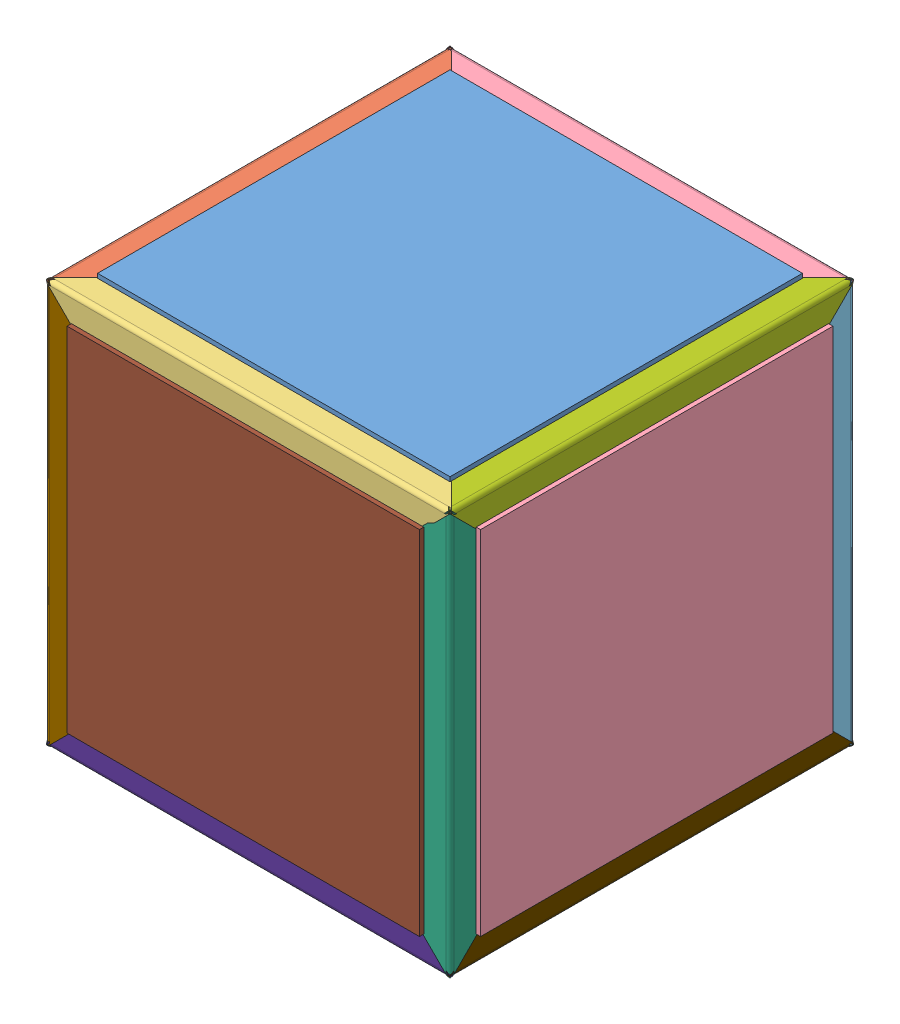
SolidWorks assembly cube_03, configuration cube03. Lengths in mm.
Overall size (150.49 150.49 150.49).
30 component instances, 30 part files, 92 mates.
Components (placement in the parent):
- pr^cube_03-28: pr^cube_03 [cube01] x (-1 0 0) z (0 0 1) size (128.27 1.59 128.27) (virtual)
- dr1^cube_03-55: dr1^cube_03 [cube01] at (-73.0546 73.66 0) x (0 -1 0) z (0 0 1) size (26.01 26.01 147.33) (virtual)
- dr2^cube_03-37: dr2^cube_03 [cube01] at (0 73.66 73.0546) x (0 -1 0) z (1 0 0) size (26.01 26.01 147.33) (virtual)
- dr3^cube_03-33: dr3^cube_03 [cube01] at (0 73.66 -73.0546) x (0 -1 0) z (-1 0 0) size (26.01 26.01 147.33) (virtual)
- br1^cube_03-49: br1^cube_03 [Default] at (0 48.26 -48.26) x (0 0 1) z (-1 0 0) size (50.8 50.8 89.41) (virtual)
- br2^cube_03-61: br2^cube_03 [Default] at (-48.26 48.26 0) size (50.8 50.8 89.41) (virtual)
- br3^cube_03-46: br3^cube_03 [Default] at (0 48.26 48.26) x (0 0 -1) z (1 0 0) size (50.8 50.8 89.41) (virtual)
- pg^cube_03-20: pg^cube_03 [cube01] x (0 -1 0) z (0 0 1) size (128.27 1.59 128.27) (virtual)
- dg1^cube_03-38: dg1^cube_03 [cube01] at (-73.66 0 73.0546) x (1 0 0) z (0 1 0) size (26.01 26.01 147.33) (virtual)
- dg2^cube_03-41: dg2^cube_03 [cube01] at (-73.66 -73.0546 0) size (26.01 26.01 147.33) (virtual)
- dg3^cube_03-34: dg3^cube_03 [cube01] at (-73.66 0 -73.0546) x (1 0 0) z (0 -1 0) size (26.01 26.01 147.33) (virtual)
- bg1^cube_03-47: bg1^cube_03 [Default] at (-48.26 -48.26 0) x (0 1 0) z (0 0 1) size (50.8 50.8 89.41) (virtual)
- bg2^cube_03-44: bg2^cube_03 [Default] at (-48.26 0 48.26) x (0 0 -1) z (0 1 0) size (50.8 50.8 89.41) (virtual)
- bg3^cube_03-40: bg3^cube_03 [Default] at (-48.26 0 -48.26) x (0 0 1) z (0 -1 0) size (50.8 50.8 89.41) (virtual)
- py^cube_03-21: py^cube_03 [cube01] at origin size (128.27 1.59 128.27) (virtual)
- dy1^cube_03-35: dy1^cube_03 [cube01] at (0 -73.66 -73.0546) x (0 1 0) z (1 0 0) size (26.01 26.01 147.33) (virtual)
- dy2^cube_03-39: dy2^cube_03 [cube01] at (0 -73.66 73.0546) x (0 1 0) z (-1 0 0) size (26.01 26.01 147.33) (virtual)
- dy3^cube_03-42: dy3^cube_03 [cube01] at (73.0546 -73.66 0) x (0 1 0) z (0 0 1) size (26.01 26.01 147.33) (virtual)
- by1^cube_03-41: by1^cube_03 [Default] at (0 -48.26 -48.26) x (0 0 1) z (1 0 0) size (50.8 50.8 89.41) (virtual)
- by2^cube_03-45: by2^cube_03 [Default] at (0 -48.26 48.26) x (0 0 -1) z (-1 0 0) size (50.8 50.8 89.41) (virtual)
- by3^cube_03-48: by3^cube_03 [Default] at (48.26 -48.26 0) x (-1 0 0) z (0 0 1) size (50.8 50.8 89.41) (virtual)
- po^cube_03-22: po^cube_03 [cube01] x (0 1 0) z (0 0 1) size (128.27 1.59 128.27) (virtual)
- do1^cube_03-36: do1^cube_03 [cube01] at (73.66 0 -73.0546) x (-1 0 0) z (0 1 0) size (26.01 26.01 147.33) (virtual)
- do2^cube_03-40: do2^cube_03 [cube01] at (73.66 0 73.0546) x (-1 0 0) z (0 -1 0) size (26.01 26.01 147.33) (virtual)
- do3^cube_03-47: do3^cube_03 [cube01] at (73.66 73.0546 0) x (-1 0 0) z (0 0 1) size (26.01 26.01 147.33) (virtual)
- bo1^cube_03-42: bo1^cube_03 [Default] at (48.26 0 -48.26) x (0 0 1) z (0 1 0) size (50.8 50.8 89.41) (virtual)
- bo2^cube_03-46: bo2^cube_03 [Default] at (48.26 0 48.26) x (0 0 -1) z (0 -1 0) size (50.8 50.8 89.41) (virtual)
- bo3^cube_03-62: bo3^cube_03 [Default] at (48.26 48.26 0) x (0 -1 0) z (0 0 1) size (50.8 50.8 89.41) (virtual)
- pc^cube_03-18: pc^cube_03 [cube01] x (-1 0 0) z (0 -1 0) size (128.27 1.59 128.27) (virtual)
- pb^cube_03-21: pb^cube_03 [cube01] x (-1 0 0) z (0 1 0) size (128.27 1.59 128.27) (virtual)
Mates (geometry in assembly coordinates):
- Coincident1: coincident anti-aligned: plane of pr^cube_03-28 through (64.135 73.66 -64.135) normal (0 -1 0); plane of br1^cube_03-49 through (-44.704 73.66 -48.26) normal (0 1 0)
- Coincident2: coincident anti-aligned: plane of pr^cube_03-28 through (64.135 73.66 -64.135) normal (0 -1 0); plane of br2^cube_03-61 through (-48.26 73.66 44.704) normal (0 1 0)
- Coincident3: coincident anti-aligned: plane of pr^cube_03-28 through (64.135 73.66 -64.135) normal (0 -1 0); plane of br3^cube_03-46 through (44.704 73.66 48.26) normal (0 1 0)
- Coincident4: coincident anti-aligned: plane of pr^cube_03-28 through (64.135 73.66 -64.135) normal (0 -1 0); plane of bo3^cube_03-62 through (48.26 73.66 44.704) normal (0 1 0)
- Coincident5: coincident anti-aligned: plane of pr^cube_03-28 through (64.135 73.66 -64.135) normal (0 -1 0); plane of dr3^cube_03-33 through (0 73.66 -146.7146) normal (0 1 0)
- Coincident6: coincident anti-aligned: plane of pr^cube_03-28 through (64.135 73.66 -64.135) normal (0 -1 0); plane of dr1^cube_03-55 through (-146.7146 73.66 0) normal (0 1 0)
- Coincident7: coincident anti-aligned: plane of pr^cube_03-28 through (64.135 73.66 -64.135) normal (0 -1 0); plane of do3^cube_03-47 through (-0.6054 73.66 0) normal (0 1 0)
- Coincident8: coincident anti-aligned: plane of pr^cube_03-28 through (64.135 73.66 -64.135) normal (0 -1 0); plane of dr2^cube_03-37 through (0 73.66 146.7146) normal (0 1 0)
- Coincident34: coincident anti-aligned: plane of pb^cube_03-21 through (64.135 -64.135 -73.66) normal (0 0 1); plane of by1^cube_03-41 through (44.704 -48.26 -73.66) normal (0 0 -1)
- Coincident35: coincident anti-aligned: plane of pb^cube_03-21 through (64.135 -64.135 -73.66) normal (0 0 1); plane of bo1^cube_03-42 through (48.26 44.704 -73.66) normal (0 0 -1)
- Coincident36: coincident anti-aligned: plane of pb^cube_03-21 through (64.135 -64.135 -73.66) normal (0 0 1); plane of br1^cube_03-49 through (-44.704 48.26 -73.66) normal (0 0 -1)
- Coincident37: coincident anti-aligned: plane of pb^cube_03-21 through (64.135 -64.135 -73.66) normal (0 0 1); plane of bg3^cube_03-40 through (-48.26 -44.704 -73.66) normal (0 0 -1)
- Coincident38: coincident anti-aligned: plane of pb^cube_03-21 through (64.135 -64.135 -73.66) normal (0 0 1); plane of dg3^cube_03-34 through (0.6054 0 -73.66) normal (0 0 -1)
- Coincident39: coincident anti-aligned: plane of pb^cube_03-21 through (64.135 -64.135 -73.66) normal (0 0 1); plane of dr3^cube_03-33 through (0 -0.6054 -73.66) normal (0 0 -1)
- Coincident40: coincident anti-aligned: plane of pb^cube_03-21 through (64.135 -64.135 -73.66) normal (0 0 1); plane of do1^cube_03-36 through (-0.6054 0 -73.66) normal (0 0 -1)
- Coincident41: coincident anti-aligned: plane of pb^cube_03-21 through (64.135 -64.135 -73.66) normal (0 0 1); plane of dy1^cube_03-35 through (0 0.6054 -73.66) normal (0 0 -1)
- Coincident42: coincident anti-aligned: plane of pc^cube_03-18 through (64.135 64.135 73.66) normal (0 0 -1); plane of bo2^cube_03-46 through (48.26 -44.704 73.66) normal (0 0 1)
- Coincident43: coincident anti-aligned: plane of pc^cube_03-18 through (64.135 64.135 73.66) normal (0 0 -1); plane of br3^cube_03-46 through (44.704 48.26 73.66) normal (0 0 1)
- Coincident44: coincident anti-aligned: plane of pc^cube_03-18 through (64.135 64.135 73.66) normal (0 0 -1); plane of bg2^cube_03-44 through (-48.26 44.704 73.66) normal (0 0 1)
- Coincident45: coincident anti-aligned: plane of pc^cube_03-18 through (64.135 64.135 73.66) normal (0 0 -1); plane of by2^cube_03-45 through (-44.704 -48.26 73.66) normal (0 0 1)
- Coincident46: coincident anti-aligned: plane of pc^cube_03-18 through (64.135 64.135 73.66) normal (0 0 -1); plane of do2^cube_03-40 through (-0.6054 0 73.66) normal (0 0 1)
- Coincident47: coincident anti-aligned: plane of pc^cube_03-18 through (64.135 64.135 73.66) normal (0 0 -1); plane of dy2^cube_03-39 through (0 0.6054 73.66) normal (0 0 1)
- Coincident48: coincident anti-aligned: plane of pc^cube_03-18 through (64.135 64.135 73.66) normal (0 0 -1); plane of dg1^cube_03-38 through (0.6054 0 73.66) normal (0 0 1)
- Coincident49: coincident anti-aligned: plane of pc^cube_03-18 through (64.135 64.135 73.66) normal (0 0 -1); plane of dr2^cube_03-37 through (0 -0.6054 73.66) normal (0 0 1)
- Coincident50: coincident anti-aligned: plane of pg^cube_03-20 through (-73.66 64.135 -64.135) normal (1 0 0); plane of bg3^cube_03-40 through (-73.66 -44.704 -48.26) normal (-1 0 0)
- Coincident51: coincident anti-aligned: plane of pg^cube_03-20 through (-73.66 64.135 -64.135) normal (1 0 0); plane of bg1^cube_03-47 through (-73.66 -48.26 44.704) normal (-1 0 0)
- Coincident52: coincident anti-aligned: plane of pg^cube_03-20 through (-73.66 64.135 -64.135) normal (1 0 0); plane of bg2^cube_03-44 through (-73.66 44.704 48.26) normal (-1 0 0)
- Coincident53: coincident anti-aligned: plane of pg^cube_03-20 through (-73.66 64.135 -64.135) normal (1 0 0); plane of dr1^cube_03-55 through (-73.66 -0.6054 0) normal (-1 0 0)
- Coincident54: coincident anti-aligned: plane of pg^cube_03-20 through (-73.66 64.135 -64.135) normal (1 0 0); plane of dg3^cube_03-34 through (-73.66 0 -146.7146) normal (-1 0 0)
- Coincident55: coincident anti-aligned: plane of pg^cube_03-20 through (-73.66 64.135 -64.135) normal (1 0 0); plane of dg2^cube_03-41 through (-73.66 -146.7146 0) normal (-1 0 0)
- Coincident56: coincident anti-aligned: plane of pg^cube_03-20 through (-73.66 64.135 -64.135) normal (1 0 0); plane of dg1^cube_03-38 through (-73.66 0 146.7146) normal (-1 0 0)
- Coincident99: coincident anti-aligned: plane of pg^cube_03-20 through (-73.66 64.135 -64.135) normal (1 0 0); plane of br2^cube_03-61 through (-73.66 48.26 44.704) normal (-1 0 0)
- Coincident57: coincident anti-aligned: plane of py^cube_03-21 through (-64.135 -73.66 -64.135) normal (0 1 0); plane of by3^cube_03-48 through (48.26 -73.66 44.704) normal (0 -1 0)
- Coincident58: coincident anti-aligned: plane of py^cube_03-21 through (-64.135 -73.66 -64.135) normal (0 1 0); plane of by2^cube_03-45 through (-44.704 -73.66 48.26) normal (0 -1 0)
- Coincident59: coincident anti-aligned: plane of py^cube_03-21 through (-64.135 -73.66 -64.135) normal (0 1 0); plane of bg1^cube_03-47 through (-48.26 -73.66 44.704) normal (0 -1 0)
- Coincident60: coincident anti-aligned: plane of py^cube_03-21 through (-64.135 -73.66 -64.135) normal (0 1 0); plane of by1^cube_03-41 through (44.704 -73.66 -48.26) normal (0 -1 0)
- Coincident61: coincident anti-aligned: plane of py^cube_03-21 through (-64.135 -73.66 -64.135) normal (0 1 0); plane of dy3^cube_03-42 through (146.7146 -73.66 0) normal (0 -1 0)
- Coincident62: coincident anti-aligned: plane of py^cube_03-21 through (-64.135 -73.66 -64.135) normal (0 1 0); plane of dy2^cube_03-39 through (0 -73.66 146.7146) normal (0 -1 0)
- Coincident63: coincident anti-aligned: plane of py^cube_03-21 through (-64.135 -73.66 -64.135) normal (0 1 0); plane of dg2^cube_03-41 through (0.6054 -73.66 0) normal (0 -1 0)
- Coincident64: coincident anti-aligned: plane of py^cube_03-21 through (-64.135 -73.66 -64.135) normal (0 1 0); plane of dy1^cube_03-35 through (0 -73.66 -146.7146) normal (0 -1 0)
- Coincident65: coincident anti-aligned: plane of po^cube_03-22 through (73.66 -64.135 -64.135) normal (-1 0 0); plane of bo1^cube_03-42 through (73.66 44.704 -48.26) normal (1 0 0)
- Coincident66: coincident anti-aligned: plane of po^cube_03-22 through (73.66 -64.135 -64.135) normal (-1 0 0); plane of by3^cube_03-48 through (73.66 -48.26 44.704) normal (1 0 0)
- Coincident67: coincident anti-aligned: plane of po^cube_03-22 through (73.66 -64.135 -64.135) normal (-1 0 0); plane of bo2^cube_03-46 through (73.66 -44.704 48.26) normal (1 0 0)
- Coincident68: coincident anti-aligned: plane of po^cube_03-22 through (73.66 -64.135 -64.135) normal (-1 0 0); plane of bo3^cube_03-62 through (73.66 48.26 44.704) normal (1 0 0)
- Coincident69: coincident anti-aligned: plane of po^cube_03-22 through (73.66 -64.135 -64.135) normal (-1 0 0); plane of do2^cube_03-40 through (73.66 0 146.7146) normal (1 0 0)
- Coincident70: coincident anti-aligned: plane of po^cube_03-22 through (73.66 -64.135 -64.135) normal (-1 0 0); plane of do3^cube_03-47 through (73.66 146.7146 0) normal (1 0 0)
- Coincident71: coincident anti-aligned: plane of po^cube_03-22 through (73.66 -64.135 -64.135) normal (-1 0 0); plane of do1^cube_03-36 through (73.66 0 -146.7146) normal (1 0 0)
- Coincident72: coincident anti-aligned: plane of po^cube_03-22 through (73.66 -64.135 -64.135) normal (-1 0 0); plane of dy3^cube_03-42 through (73.66 0.6054 0) normal (1 0 0)
- Coincident73: coincident aligned: plane of assembly through (0 0 0) normal (0 0 1); plane of dy3^cube_03-42 through (73.0546 -73.66 0) normal (0 0 1)
- Coincident74: coincident aligned: plane of assembly through (0 0 0) normal (0 0 1); plane of by3^cube_03-48 through (48.26 -48.26 0) normal (0 0 1)
- Coincident75: coincident aligned: plane of assembly through (0 0 0) normal (0 0 1); plane of bo3^cube_03-62 through (48.26 48.26 0) normal (0 0 1)
- Coincident76: coincident aligned: plane of assembly through (0 0 0) normal (0 0 1); plane of do3^cube_03-47 through (73.66 73.0546 0) normal (0 0 1)
- Coincident77: coincident aligned: plane of assembly through (0 0 0) normal (0 0 1); plane of dg2^cube_03-41 through (-73.66 -73.0546 0) normal (0 0 1)
- Coincident78: coincident aligned: plane of assembly through (0 0 0) normal (0 0 1); plane of bg1^cube_03-47 through (-48.26 -48.26 0) normal (0 0 1)
- Coincident79: coincident aligned: plane of assembly through (0 0 0) normal (0 0 1); plane of dr1^cube_03-55 through (-73.0546 73.66 0) normal (0 0 1)
- Coincident80: coincident aligned: plane of assembly through (0 0 0) normal (0 0 1); plane of br2^cube_03-61 through (-48.26 48.26 0) normal (0 0 1)
- Coincident81: coincident aligned: plane of assembly through (0 0 0) normal (0 1 0); plane of bo1^cube_03-42 through (48.26 0 -48.26) normal (0 1 0)
- Coincident82: coincident aligned: plane of assembly through (0 0 0) normal (0 1 0); plane of py^cube_03-21 through (0 0 0) normal (0 1 0)
- Coincident83: coincident aligned: plane of assembly through (0 0 0) normal (0 1 0); plane of do1^cube_03-36 through (73.66 0 -73.0546) normal (0 1 0)
- Coincident84: coincident anti-aligned: plane of assembly through (0 0 0) normal (0 1 0); plane of bg3^cube_03-40 through (-48.26 0 -48.26) normal (0 -1 0)
- Coincident85: coincident anti-aligned: plane of assembly through (0 0 0) normal (0 1 0); plane of dg3^cube_03-34 through (-73.66 0 -73.0546) normal (0 -1 0)
- Coincident86: coincident aligned: plane of assembly through (0 0 0) normal (0 1 0); plane of dg1^cube_03-38 through (-73.66 0 73.0546) normal (0 1 0)
- Coincident87: coincident aligned: plane of assembly through (0 0 0) normal (0 1 0); plane of bg2^cube_03-44 through (-48.26 0 48.26) normal (0 1 0)
- Coincident88: coincident anti-aligned: plane of assembly through (0 0 0) normal (0 1 0); plane of bo2^cube_03-46 through (48.26 0 48.26) normal (0 -1 0)
- Coincident89: coincident anti-aligned: plane of assembly through (0 0 0) normal (0 1 0); plane of do2^cube_03-40 through (73.66 0 73.0546) normal (0 -1 0)
- Coincident90: coincident anti-aligned: plane of assembly through (0 0 0) normal (1 0 0); plane of by2^cube_03-45 through (0 -48.26 48.26) normal (-1 0 0)
- Coincident91: coincident anti-aligned: plane of assembly through (0 0 0) normal (1 0 0); plane of dy2^cube_03-39 through (0 -73.66 73.0546) normal (-1 0 0)
- Coincident92: coincident aligned: plane of assembly through (0 0 0) normal (1 0 0); plane of pg^cube_03-20
- Coincident93: coincident aligned: plane of assembly through (0 0 0) normal (1 0 0); plane of dr2^cube_03-37 through (0 73.66 73.0546) normal (1 0 0)
- Coincident94: coincident aligned: plane of assembly through (0 0 0) normal (1 0 0); plane of br3^cube_03-46 through (0 48.26 48.26) normal (1 0 0)
- Coincident95: coincident anti-aligned: plane of assembly through (0 0 0) normal (1 0 0); plane of dr3^cube_03-33 through (0 73.66 -73.0546) normal (-1 0 0)
- Coincident96: coincident anti-aligned: plane of assembly through (0 0 0) normal (1 0 0); plane of br1^cube_03-49 through (0 48.26 -48.26) normal (-1 0 0)
- Coincident97: coincident aligned: plane of assembly through (0 0 0) normal (1 0 0); plane of by1^cube_03-41 through (0 -48.26 -48.26) normal (1 0 0)
- Coincident98: coincident aligned: plane of assembly through (0 0 0) normal (1 0 0); plane of dy1^cube_03-35 through (0 -73.66 -73.0546) normal (1 0 0)
- Coincident100: coincident anti-aligned: plane of pr^cube_03-28; plane of assembly through (0 0 0) normal (1 0 0)
- Coincident101: coincident aligned: plane of pr^cube_03-28 through (0 0 0) normal (0 0 1); plane of assembly through (0 0 0) normal (0 0 1)
- Coincident102: coincident anti-aligned: plane of pr^cube_03-28; plane of assembly through (0 0 0) normal (0 1 0)
- Coincident106: coincident anti-aligned: plane of pg^cube_03-20; plane of assembly through (0 0 0) normal (0 1 0)
- Coincident107: coincident aligned: plane of pg^cube_03-20; plane of assembly through (0 0 0) normal (1 0 0)
- Coincident108: coincident aligned: plane of pg^cube_03-20 through (0 0 0) normal (0 0 1); plane of assembly through (0 0 0) normal (0 0 1)
- Coincident109: coincident aligned: plane of py^cube_03-21 through (0 0 0) normal (0 0 1); plane of assembly through (0 0 0) normal (0 0 1)
- Coincident110: coincident aligned: plane of py^cube_03-21 through (0 0 0) normal (0 1 0); plane of assembly through (0 0 0) normal (0 1 0)
- Coincident111: coincident aligned: plane of py^cube_03-21 through (0 0 0) normal (1 0 0); plane of assembly through (0 0 0) normal (1 0 0)
- Coincident112: coincident aligned: plane of po^cube_03-22 through (0 0 0) normal (0 0 1); plane of assembly through (0 0 0) normal (0 0 1)
- Coincident113: coincident anti-aligned: plane of po^cube_03-22; plane of assembly through (0 0 0) normal (1 0 0)
- Coincident114: coincident aligned: plane of po^cube_03-22; plane of assembly through (0 0 0) normal (0 1 0)
- Coincident115: coincident anti-aligned: plane of pc^cube_03-18 through (0 0 0) normal (0 -1 0); plane of assembly through (0 0 0) normal (0 1 0)
- Coincident116: coincident anti-aligned: plane of pc^cube_03-18; plane of assembly through (0 0 0) normal (0 0 1)
- Coincident117: coincident anti-aligned: plane of pc^cube_03-18; plane of assembly through (0 0 0) normal (1 0 0)
- Coincident118: coincident aligned: plane of pb^cube_03-21 through (0 0 0) normal (0 1 0); plane of assembly through (0 0 0) normal (0 1 0)
- Coincident119: coincident aligned: plane of pb^cube_03-21; plane of assembly through (0 0 0) normal (0 0 1)
- Coincident120: coincident anti-aligned: line of pb^cube_03-21 through (0.8731 -0.8731 0) axis (0 0 -1); plane of assembly through (0 0 0) normal (1 0 0)
